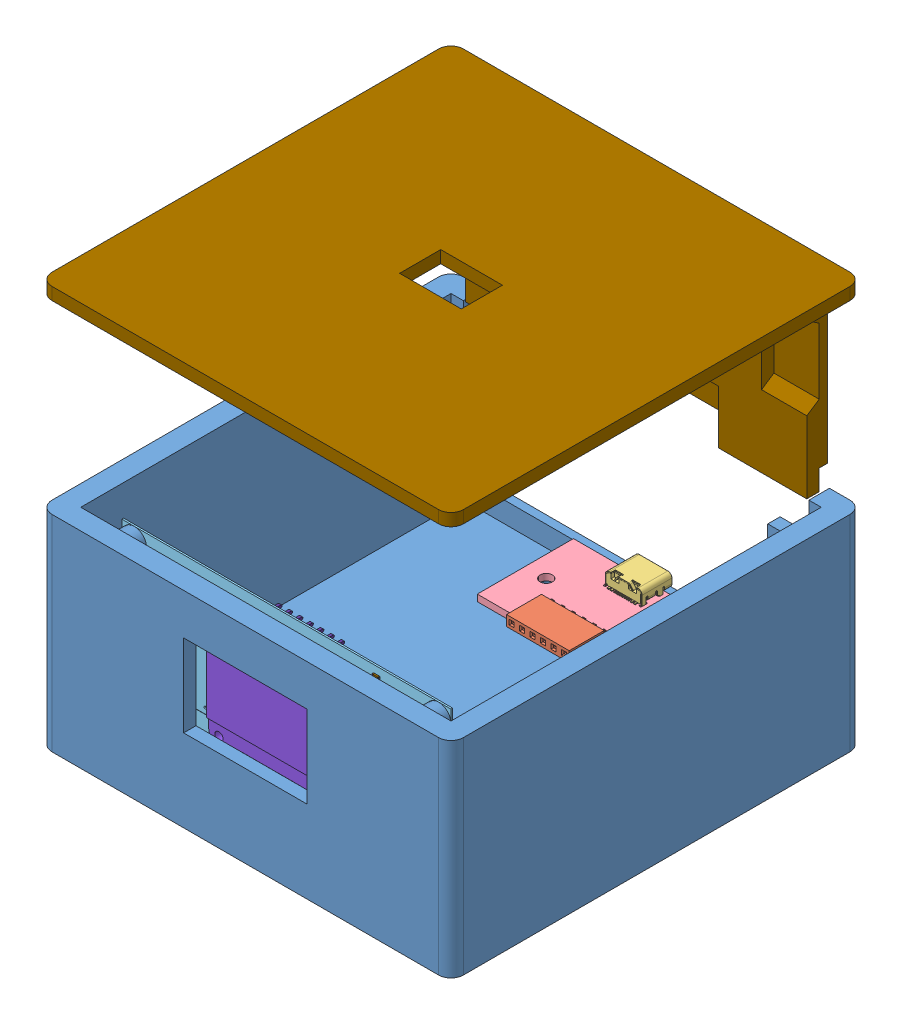
SolidWorks assembly 提醒喝水器, configuration 默认. Lengths in mm.
Overall size (100 98 100).
295 component instances, 117 part files, 15 mates.
Components (placement in the parent):
- 外壳-1: 外壳 [默认] at (-140.6896 -46.2345 50) size (100 50 100)
- Type-C_Ext-1: Type-C_Ext [默认] at (-1.1691 -37.2345 -151.062) x (0 0 1) z (0 1 0) size (28.17 35.81 6.47)
  - Type-C_Ext(2)^Type-C_Ext-1: Type-C_Ext(2)^Type-C_Ext [默认] at origin size (28.17 35.81 6.47) (virtual)
    - PinSocket_1x06_P2.54mm_Horizontal^Type-C_Ext(2)_Type-C_Ext-1: PinSocket_1x06_P2.54mm_Horizontal^Type-C_Ext(2)_Type-C_Ext [默认] at (120.06 -95.733 1.65) x (-1 0 0) z (0 0 1) size (10.13 15.24 5.84) (virtual)
      - SOLID^PinSocket_1x06_P2.54mm_Horizontal_Type-C_Ext(2)_Type-C_Ext-1: SOLID^PinSocket_1x06_P2.54mm_Horizontal_Type-C_Ext(2)_Type-C_Ext [默认] at origin size (10.13 15.24 5.84) (virtual)
    - Type-C_16Pin_ThroughtHole^Type-C_Ext(2)_Type-C_Ext-1: Type-C_16Pin_ThroughtHole^Type-C_Ext(2)_Type-C_Ext [默认] at (106.934 -89.408 0.126) x (0 -1 0) z (0 0 1) size (8.94 7.9 4.1) (virtual)
      - COMPOUND^Type-C_16Pin_ThroughtHole_Type-C_Ext(2)_Type-C_Ext-1: COMPOUND^Type-C_16Pin_ThroughtHole_Type-C_Ext(2)_Type-C_Ext [默认] at origin size (8.94 7.9 4.1) (virtual)
    - Type-C_Ext PCB^Type-C_Ext(2)_Type-C_Ext-1: Type-C_Ext PCB^Type-C_Ext(2)_Type-C_Ext [默认] at origin size (23.37 35.81 1.6) (virtual)
- MainBoard-1: MainBoard [默认] at (-130.6896 -38.7345 40) size (80 40 10.66)
  - MainBoard(2)^MainBoard-1: MainBoard(2)^MainBoard [默认] at origin size (80 40 10.66) (virtual)
    - Board^MainBoard(2)_MainBoard-1: Board^MainBoard(2)_MainBoard [默认] at origin size (80 40 0.41) (virtual)
      - Open CASCADE STEP translator 6.8 1.1.1^Board_MainBoard(2)_MainBoard-1: Open CASCADE STEP translator 6.8 1.1.1^Board_MainBoard(2)_MainBoard [默认] at (0 0 -0.4115) size (80 40 0.41) (virtual)
    - LS1^MainBoard(2)_MainBoard-1: LS1^MainBoard(2)_MainBoard [默认] at origin size (9 9 9) (virtual)
      - BEEP_5x9x5.5^LS1_MainBoard(2)_MainBoard-1: BEEP_5x9x5.5^LS1_MainBoard(2)_MainBoard [默认] at (40.0051 20.0659 -0.4115) x (1 0 0) z (0 0 -1) size (9 9 9) (virtual)
        - BEEP_5X9X5_5-3924_AF0_ASM^BEEP_5x9x5.5_LS1_MainBoard(2)_MainBoard-1: BEEP_5X9X5_5-3924_AF0_ASM^BEEP_5x9x5.5_LS1_MainBoard(2)_MainBoard [默认] at origin size (9 9 9) (virtual)
          - BEEP_5X9X5_5-6370_AF0^BEEP_5X9X5_5-3924_AF0_ASM_BEEP_5x9x5.5_LS1_MainBoard(2)_MainBoard-1: BEEP_5X9X5_5-6370_AF0^BEEP_5X9X5_5-3924_AF0_ASM_BEEP_5x9x5.5_LS1_MainBoard(2)_MainBoard [默认] at origin size (9 9 9) (virtual)
    - X1^MainBoard(2)_MainBoard-1: X1^MainBoard(2)_MainBoard [默认] at origin size (2.5 3.2 0.72) (virtual)
      - OSC_3225-4^X1_MainBoard(2)_MainBoard-1: OSC_3225-4^X1_MainBoard(2)_MainBoard [默认] at (73.6601 29.4639 0) x (0 -1 0) z (0 0 1) size (3.2 2.5 0.72) (virtual)
        - OSC_3225-4-6525_AF0_ASM^OSC_3225-4_X1_MainBoard(2)_MainBoard-1: OSC_3225-4-6525_AF0_ASM^OSC_3225-4_X1_MainBoard(2)_MainBoard [默认] at origin size (3.2 2.5 0.72) (virtual)
          - OSC_3225-4-11675_AF0_ASM^OSC_3225-4-6525_AF0_ASM_OSC_3225-4_X1_MainBoard(2)_MainBoard-1: OSC_3225-4-11675_AF0_ASM^OSC_3225-4-6525_AF0_ASM_OSC_3225-4_X1_MainBoard(2)_MainBoard [默认] at origin size (3.2 2.5 0.72) (virtual)
            - _3_1_20001^OSC_3225-4-11675_AF0_ASM_OSC_3225-4-6525_AF0_ASM_OSC_3225-4_X1_MainBoard(2)_MainBoard-1: _3_1_20001^OSC_3225-4-11675_AF0_ASM_OSC_3225-4-6525_AF0_ASM_OSC_3225-4_X1_MainBoard(2)_MainBoard [默认] at origin size (3.08 2.38 0.23) (virtual)
            - _4_4__1_20001^OSC_3225-4-11675_AF0_ASM_OSC_3225-4-6525_AF0_ASM_OSC_3225-4_X1_MainBoard(2)_MainBoard-1: _4_4__1_20001^OSC_3225-4-11675_AF0_ASM_OSC_3225-4-6525_AF0_ASM_OSC_3225-4_X1_MainBoard(2)_MainBoard [默认] at origin size (1 0.9 0.02) (virtual)
            - _4_2__1_20001^OSC_3225-4-11675_AF0_ASM_OSC_3225-4-6525_AF0_ASM_OSC_3225-4_X1_MainBoard(2)_MainBoard-1: _4_2__1_20001^OSC_3225-4-11675_AF0_ASM_OSC_3225-4-6525_AF0_ASM_OSC_3225-4_X1_MainBoard(2)_MainBoard [默认] at origin size (1 0.9 0.02) (virtual)
            - _4_1__1_20001^OSC_3225-4-11675_AF0_ASM_OSC_3225-4-6525_AF0_ASM_OSC_3225-4_X1_MainBoard(2)_MainBoard-1: _4_1__1_20001^OSC_3225-4-11675_AF0_ASM_OSC_3225-4-6525_AF0_ASM_OSC_3225-4_X1_MainBoard(2)_MainBoard [默认] at origin size (1 0.9 0.02) (virtual)
            - _4_3__1_20001^OSC_3225-4-11675_AF0_ASM_OSC_3225-4-6525_AF0_ASM_OSC_3225-4_X1_MainBoard(2)_MainBoard-1: _4_3__1_20001^OSC_3225-4-11675_AF0_ASM_OSC_3225-4-6525_AF0_ASM_OSC_3225-4_X1_MainBoard(2)_MainBoard [默认] at origin size (1 0.9 0.02) (virtual)
            - _2_1_2_AF0^OSC_3225-4-11675_AF0_ASM_OSC_3225-4-6525_AF0_ASM_OSC_3225-4_X1_MainBoard(2)_MainBoard-1: _2_1_2_AF0^OSC_3225-4-11675_AF0_ASM_OSC_3225-4-6525_AF0_ASM_OSC_3225-4_X1_MainBoard(2)_MainBoard [默认] at origin size (3.2 2.5 0.47) (virtual)
    - U2^MainBoard(2)_MainBoard-1: U2^MainBoard(2)_MainBoard [默认] at origin size (2.81 3 1.18) (virtual)
      - SOT23-6^U2_MainBoard(2)_MainBoard-1: SOT23-6^U2_MainBoard(2)_MainBoard [默认] at (55.1181 16.1291 0) x (0 -1 0) z (0 0 1) size (3 2.81 1.18) (virtual)
        - SOT23-6-13550_AF0_ASM^SOT23-6_U2_MainBoard(2)_MainBoard-1: SOT23-6-13550_AF0_ASM^SOT23-6_U2_MainBoard(2)_MainBoard [默认] at origin size (3 2.81 1.18) (virtual)
          - SOT23-5AND6__100^SOT23-6-13550_AF0_ASM_SOT23-6_U2_MainBoard(2)_MainBoard-1: SOT23-5AND6__100^SOT23-6-13550_AF0_ASM_SOT23-6_U2_MainBoard(2)_MainBoard [默认] at (0.95 0.8 0.675) size (0.4 0.6 0.78) (virtual)
          - SOT23-5AND6__100^SOT23-6-13550_AF0_ASM_SOT23-6_U2_MainBoard(2)_MainBoard-2: SOT23-5AND6__100^SOT23-6-13550_AF0_ASM_SOT23-6_U2_MainBoard(2)_MainBoard [默认] at (-0.95 -0.8 0.675) x (-1 0 0) z (0 0 1) size (0.4 0.6 0.78) (virtual)
          - SOT23-6-7933_AF0^SOT23-6-13550_AF0_ASM_SOT23-6_U2_MainBoard(2)_MainBoard-1: SOT23-6-7933_AF0^SOT23-6-13550_AF0_ASM_SOT23-6_U2_MainBoard(2)_MainBoard [默认] at origin size (3 1.6 1.1) (virtual)
          - SOT23-5AND6__100^SOT23-6-13550_AF0_ASM_SOT23-6_U2_MainBoard(2)_MainBoard-3: SOT23-5AND6__100^SOT23-6-13550_AF0_ASM_SOT23-6_U2_MainBoard(2)_MainBoard [默认] at (0 -0.8 0.675) x (-1 0 0) z (0 0 1) size (0.4 0.6 0.78) (virtual)
          - SOT23-5AND6__100^SOT23-6-13550_AF0_ASM_SOT23-6_U2_MainBoard(2)_MainBoard-4: SOT23-5AND6__100^SOT23-6-13550_AF0_ASM_SOT23-6_U2_MainBoard(2)_MainBoard [默认] at (0 0.8 0.675) size (0.4 0.6 0.78) (virtual)
          - SOT23-5AND6__100^SOT23-6-13550_AF0_ASM_SOT23-6_U2_MainBoard(2)_MainBoard-5: SOT23-5AND6__100^SOT23-6-13550_AF0_ASM_SOT23-6_U2_MainBoard(2)_MainBoard [默认] at (0.95 -0.8 0.675) x (-1 0 0) z (0 0 1) size (0.4 0.6 0.78) (virtual)
          - SOT23-5AND6__100^SOT23-6-13550_AF0_ASM_SOT23-6_U2_MainBoard(2)_MainBoard-6: SOT23-5AND6__100^SOT23-6-13550_AF0_ASM_SOT23-6_U2_MainBoard(2)_MainBoard [默认] at (-0.95 0.8 0.675) size (0.4 0.6 0.78) (virtual)
    - U1^MainBoard(2)_MainBoard-1: U1^MainBoard(2)_MainBoard [默认] at origin size (10.01 6.01 1.9) (virtual)
      - SOP16^U1_MainBoard(2)_MainBoard-1: SOP16^U1_MainBoard(2)_MainBoard [默认] at (65.913 29.7181 0) x (0 1 0) z (0 0 1) size (6.01 10.01 1.9) (virtual)
        - SOP16_1_AF0_ASM^SOP16_U1_MainBoard(2)_MainBoard-1: SOP16_1_AF0_ASM^SOP16_U1_MainBoard(2)_MainBoard [默认] at origin size (6.01 10.01 1.9) (virtual)
          - 1_8__10001^SOP16_1_AF0_ASM_SOP16_U1_MainBoard(2)_MainBoard-1: 1_8__10001^SOP16_1_AF0_ASM_SOP16_U1_MainBoard(2)_MainBoard [默认] at (-1.8 -4.44 1) x (0 -1 0) z (0 0 1) size (0.5 1.2 1.1) (virtual)
          - 1_8__10001^SOP16_1_AF0_ASM_SOP16_U1_MainBoard(2)_MainBoard-2: 1_8__10001^SOP16_1_AF0_ASM_SOP16_U1_MainBoard(2)_MainBoard [默认] at (1.8 -0.63 1) x (0 1 0) z (0 0 1) size (0.5 1.2 1.1) (virtual)
          - 1_8__10001^SOP16_1_AF0_ASM_SOP16_U1_MainBoard(2)_MainBoard-3: 1_8__10001^SOP16_1_AF0_ASM_SOP16_U1_MainBoard(2)_MainBoard [默认] at (-1.8 1.91 1) x (0 -1 0) z (0 0 1) size (0.5 1.2 1.1) (virtual)
          - SOP16__A^SOP16_1_AF0_ASM_SOP16_U1_MainBoard(2)_MainBoard-1: SOP16__A^SOP16_1_AF0_ASM_SOP16_U1_MainBoard(2)_MainBoard [默认] at origin size (3.61 10.01 1.8) (virtual)
          - 1_8__10001^SOP16_1_AF0_ASM_SOP16_U1_MainBoard(2)_MainBoard-4: 1_8__10001^SOP16_1_AF0_ASM_SOP16_U1_MainBoard(2)_MainBoard [默认] at (1.8 -1.9 1) x (0 1 0) z (0 0 1) size (0.5 1.2 1.1) (virtual)
          - 1_8__10001^SOP16_1_AF0_ASM_SOP16_U1_MainBoard(2)_MainBoard-5: 1_8__10001^SOP16_1_AF0_ASM_SOP16_U1_MainBoard(2)_MainBoard [默认] at (-1.8 0.64 1) x (0 -1 0) z (0 0 1) size (0.5 1.2 1.1) (virtual)
          - 1_8__10001^SOP16_1_AF0_ASM_SOP16_U1_MainBoard(2)_MainBoard-6: 1_8__10001^SOP16_1_AF0_ASM_SOP16_U1_MainBoard(2)_MainBoard [默认] at (1.8 4.45 1) x (0 1 0) z (0 0 1) size (0.5 1.2 1.1) (virtual)
          - 1_8__10001^SOP16_1_AF0_ASM_SOP16_U1_MainBoard(2)_MainBoard-7: 1_8__10001^SOP16_1_AF0_ASM_SOP16_U1_MainBoard(2)_MainBoard [默认] at (1.8 -3.17 1) x (0 1 0) z (0 0 1) size (0.5 1.2 1.1) (virtual)
          - 1_8__10001^SOP16_1_AF0_ASM_SOP16_U1_MainBoard(2)_MainBoard-8: 1_8__10001^SOP16_1_AF0_ASM_SOP16_U1_MainBoard(2)_MainBoard [默认] at (-1.8 -0.63 1) x (0 -1 0) z (0 0 1) size (0.5 1.2 1.1) (virtual)
          - 1_8__10001^SOP16_1_AF0_ASM_SOP16_U1_MainBoard(2)_MainBoard-9: 1_8__10001^SOP16_1_AF0_ASM_SOP16_U1_MainBoard(2)_MainBoard [默认] at (1.8 3.18 1) x (0 1 0) z (0 0 1) size (0.5 1.2 1.1) (virtual)
          - 1_8__10001^SOP16_1_AF0_ASM_SOP16_U1_MainBoard(2)_MainBoard-10: 1_8__10001^SOP16_1_AF0_ASM_SOP16_U1_MainBoard(2)_MainBoard [默认] at (1.8 -4.44 1) x (0 1 0) z (0 0 1) size (0.5 1.2 1.1) (virtual)
          - 1_8__10001^SOP16_1_AF0_ASM_SOP16_U1_MainBoard(2)_MainBoard-11: 1_8__10001^SOP16_1_AF0_ASM_SOP16_U1_MainBoard(2)_MainBoard [默认] at (-1.8 -1.9 1) x (0 -1 0) z (0 0 1) size (0.5 1.2 1.1) (virtual)
          - 1_8__10001^SOP16_1_AF0_ASM_SOP16_U1_MainBoard(2)_MainBoard-12: 1_8__10001^SOP16_1_AF0_ASM_SOP16_U1_MainBoard(2)_MainBoard [默认] at (1.8 1.91 1) x (0 1 0) z (0 0 1) size (0.5 1.2 1.1) (virtual)
          - 1_8__10001^SOP16_1_AF0_ASM_SOP16_U1_MainBoard(2)_MainBoard-13: 1_8__10001^SOP16_1_AF0_ASM_SOP16_U1_MainBoard(2)_MainBoard [默认] at (-1.8 4.45 1) x (0 -1 0) z (0 0 1) size (0.5 1.2 1.1) (virtual)
          - 1_8__10001^SOP16_1_AF0_ASM_SOP16_U1_MainBoard(2)_MainBoard-14: 1_8__10001^SOP16_1_AF0_ASM_SOP16_U1_MainBoard(2)_MainBoard [默认] at (-1.8 -3.17 1) x (0 -1 0) z (0 0 1) size (0.5 1.2 1.1) (virtual)
          - 1_8__10001^SOP16_1_AF0_ASM_SOP16_U1_MainBoard(2)_MainBoard-15: 1_8__10001^SOP16_1_AF0_ASM_SOP16_U1_MainBoard(2)_MainBoard [默认] at (1.8 0.64 1) x (0 1 0) z (0 0 1) size (0.5 1.2 1.1) (virtual)
          - 1_8__10001^SOP16_1_AF0_ASM_SOP16_U1_MainBoard(2)_MainBoard-16: 1_8__10001^SOP16_1_AF0_ASM_SOP16_U1_MainBoard(2)_MainBoard [默认] at (-1.8 3.18 1) x (0 -1 0) z (0 0 1) size (0.5 1.2 1.1) (virtual)
    - R11^MainBoard(2)_MainBoard-1: R11^MainBoard(2)_MainBoard [默认] at origin size (1.6 0.8 0.4) (virtual)
      - 0603^R11_MainBoard(2)_MainBoard-1: 0603^R11_MainBoard(2)_MainBoard [默认] at (53.213 12.0651 0) x (1 0 0) z (0 0 1) size (1.6 0.8 0.4) (virtual)
        - R_0603-3615_AF0_ASM^0603_R11_MainBoard(2)_MainBoard-1: R_0603-3615_AF0_ASM^0603_R11_MainBoard(2)_MainBoard [默认] at origin size (1.6 0.8 0.4) (virtual)
          - R_0603-3601_AF0_ASM^R_0603-3615_AF0_ASM_0603_R11_MainBoard(2)_MainBoard-1: R_0603-3601_AF0_ASM^R_0603-3615_AF0_ASM_0603_R11_MainBoard(2)_MainBoard [默认] at origin size (1.6 0.8 0.4) (virtual)
            - _2_1_2_3_4_5_60001^R_0603-3601_AF0_ASM_R_0603-3615_AF0_ASM_0603_R11_MainBoard(2)_MainBoard-1: _2_1_2_3_4_5_60001^R_0603-3601_AF0_ASM_R_0603-3615_AF0_ASM_0603_R11_MainBoard(2)_MainBoard [默认] at origin size (0.25 0.8 0.4) (virtual)
            - _7_1_2_3_AF0^R_0603-3601_AF0_ASM_R_0603-3615_AF0_ASM_0603_R11_MainBoard(2)_MainBoard-1: _7_1_2_3_AF0^R_0603-3601_AF0_ASM_R_0603-3615_AF0_ASM_0603_R11_MainBoard(2)_MainBoard [默认] at origin size (1.5 0.8 0.4) (virtual)
            - 5_1_2_3_4_5_600^R_0603-3601_AF0_ASM_R_0603-3615_AF0_ASM_0603_R11_MainBoard(2)_MainBoard-1: 5_1_2_3_4_5_600^R_0603-3601_AF0_ASM_R_0603-3615_AF0_ASM_0603_R11_MainBoard(2)_MainBoard [默认] at origin size (0.25 0.8 0.4) (virtual)
    - R10^MainBoard(2)_MainBoard-1: R10^MainBoard(2)_MainBoard [默认] at origin size (1.6 0.8 0.4) (virtual)
      - 0603^R10_MainBoard(2)_MainBoard-1: 0603^R10_MainBoard(2)_MainBoard [默认] at (58.928 14.9861 0) x (1 0 0) z (0 0 1) size (1.6 0.8 0.4) (virtual)
        - R_0603-3615_AF0_ASM^0603_R10_MainBoard(2)_MainBoard-1: R_0603-3615_AF0_ASM^0603_R10_MainBoard(2)_MainBoard [默认] at origin size (1.6 0.8 0.4) (virtual)
          - R_0603-3601_AF0_ASM^R_0603-3615_AF0_ASM_0603_R10_MainBoard(2)_MainBoard-1: R_0603-3601_AF0_ASM^R_0603-3615_AF0_ASM_0603_R10_MainBoard(2)_MainBoard [默认] at origin size (1.6 0.8 0.4) (virtual)
            - _2_1_2_3_4_5_60001^R_0603-3601_AF0_ASM_R_0603-3615_AF0_ASM_0603_R10_MainBoard(2)_MainBoard-1: _2_1_2_3_4_5_60001^R_0603-3601_AF0_ASM_R_0603-3615_AF0_ASM_0603_R10_MainBoard(2)_MainBoard [默认] at origin size (0.25 0.8 0.4) (virtual)
            - _7_1_2_3_AF0^R_0603-3601_AF0_ASM_R_0603-3615_AF0_ASM_0603_R10_MainBoard(2)_MainBoard-1: _7_1_2_3_AF0^R_0603-3601_AF0_ASM_R_0603-3615_AF0_ASM_0603_R10_MainBoard(2)_MainBoard [默认] at origin size (1.5 0.8 0.4) (virtual)
            - 5_1_2_3_4_5_600^R_0603-3601_AF0_ASM_R_0603-3615_AF0_ASM_0603_R10_MainBoard(2)_MainBoard-1: 5_1_2_3_4_5_600^R_0603-3601_AF0_ASM_R_0603-3615_AF0_ASM_0603_R10_MainBoard(2)_MainBoard [默认] at origin size (0.25 0.8 0.4) (virtual)
    - R9^MainBoard(2)_MainBoard-1: R9^MainBoard(2)_MainBoard [默认] at origin size (1.6 0.8 0.4) (virtual)
      - 0603^R9_MainBoard(2)_MainBoard-1: 0603^R9_MainBoard(2)_MainBoard [默认] at (53.2281 10.0332 0) x (1 0 0) z (0 0 1) size (1.6 0.8 0.4) (virtual)
        - R_0603-3615_AF0_ASM^0603_R9_MainBoard(2)_MainBoard-1: R_0603-3615_AF0_ASM^0603_R9_MainBoard(2)_MainBoard [默认] at origin size (1.6 0.8 0.4) (virtual)
          - R_0603-3601_AF0_ASM^R_0603-3615_AF0_ASM_0603_R9_MainBoard(2)_MainBoard-1: R_0603-3601_AF0_ASM^R_0603-3615_AF0_ASM_0603_R9_MainBoard(2)_MainBoard [默认] at origin size (1.6 0.8 0.4) (virtual)
            - _2_1_2_3_4_5_60001^R_0603-3601_AF0_ASM_R_0603-3615_AF0_ASM_0603_R9_MainBoard(2)_MainBoard-1: _2_1_2_3_4_5_60001^R_0603-3601_AF0_ASM_R_0603-3615_AF0_ASM_0603_R9_MainBoard(2)_MainBoard [默认] at origin size (0.25 0.8 0.4) (virtual)
            - _7_1_2_3_AF0^R_0603-3601_AF0_ASM_R_0603-3615_AF0_ASM_0603_R9_MainBoard(2)_MainBoard-1: _7_1_2_3_AF0^R_0603-3601_AF0_ASM_R_0603-3615_AF0_ASM_0603_R9_MainBoard(2)_MainBoard [默认] at origin size (1.5 0.8 0.4) (virtual)
            - 5_1_2_3_4_5_600^R_0603-3601_AF0_ASM_R_0603-3615_AF0_ASM_0603_R9_MainBoard(2)_MainBoard-1: 5_1_2_3_4_5_600^R_0603-3601_AF0_ASM_R_0603-3615_AF0_ASM_0603_R9_MainBoard(2)_MainBoard [默认] at origin size (0.25 0.8 0.4) (virtual)
    - R8^MainBoard(2)_MainBoard-1: R8^MainBoard(2)_MainBoard [默认] at origin size (1.6 0.8 0.4) (virtual)
      - 0603^R8_MainBoard(2)_MainBoard-1: 0603^R8_MainBoard(2)_MainBoard [默认] at (61.976 37.8461 0) x (1 0 0) z (0 0 1) size (1.6 0.8 0.4) (virtual)
        - R_0603-3615_AF0_ASM^0603_R8_MainBoard(2)_MainBoard-1: R_0603-3615_AF0_ASM^0603_R8_MainBoard(2)_MainBoard [默认] at origin size (1.6 0.8 0.4) (virtual)
          - R_0603-3601_AF0_ASM^R_0603-3615_AF0_ASM_0603_R8_MainBoard(2)_MainBoard-1: R_0603-3601_AF0_ASM^R_0603-3615_AF0_ASM_0603_R8_MainBoard(2)_MainBoard [默认] at origin size (1.6 0.8 0.4) (virtual)
            - _2_1_2_3_4_5_60001^R_0603-3601_AF0_ASM_R_0603-3615_AF0_ASM_0603_R8_MainBoard(2)_MainBoard-1: _2_1_2_3_4_5_60001^R_0603-3601_AF0_ASM_R_0603-3615_AF0_ASM_0603_R8_MainBoard(2)_MainBoard [默认] at origin size (0.25 0.8 0.4) (virtual)
            - _7_1_2_3_AF0^R_0603-3601_AF0_ASM_R_0603-3615_AF0_ASM_0603_R8_MainBoard(2)_MainBoard-1: _7_1_2_3_AF0^R_0603-3601_AF0_ASM_R_0603-3615_AF0_ASM_0603_R8_MainBoard(2)_MainBoard [默认] at origin size (1.5 0.8 0.4) (virtual)
            - 5_1_2_3_4_5_600^R_0603-3601_AF0_ASM_R_0603-3615_AF0_ASM_0603_R8_MainBoard(2)_MainBoard-1: 5_1_2_3_4_5_600^R_0603-3601_AF0_ASM_R_0603-3615_AF0_ASM_0603_R8_MainBoard(2)_MainBoard [默认] at origin size (0.25 0.8 0.4) (virtual)
    - R7^MainBoard(2)_MainBoard-1: R7^MainBoard(2)_MainBoard [默认] at origin size (0.8 1.6 0.4) (virtual)
      - 0603^R7_MainBoard(2)_MainBoard-1: 0603^R7_MainBoard(2)_MainBoard [默认] at (10.5411 7.62 0) x (0 -1 0) z (0 0 1) size (1.6 0.8 0.4) (virtual)
        - R_0603-3615_AF0_ASM^0603_R7_MainBoard(2)_MainBoard-1: R_0603-3615_AF0_ASM^0603_R7_MainBoard(2)_MainBoard [默认] at origin size (1.6 0.8 0.4) (virtual)
          - R_0603-3601_AF0_ASM^R_0603-3615_AF0_ASM_0603_R7_MainBoard(2)_MainBoard-1: R_0603-3601_AF0_ASM^R_0603-3615_AF0_ASM_0603_R7_MainBoard(2)_MainBoard [默认] at origin size (1.6 0.8 0.4) (virtual)
            - _2_1_2_3_4_5_60001^R_0603-3601_AF0_ASM_R_0603-3615_AF0_ASM_0603_R7_MainBoard(2)_MainBoard-1: _2_1_2_3_4_5_60001^R_0603-3601_AF0_ASM_R_0603-3615_AF0_ASM_0603_R7_MainBoard(2)_MainBoard [默认] at origin size (0.25 0.8 0.4) (virtual)
            - _7_1_2_3_AF0^R_0603-3601_AF0_ASM_R_0603-3615_AF0_ASM_0603_R7_MainBoard(2)_MainBoard-1: _7_1_2_3_AF0^R_0603-3601_AF0_ASM_R_0603-3615_AF0_ASM_0603_R7_MainBoard(2)_MainBoard [默认] at origin size (1.5 0.8 0.4) (virtual)
            - 5_1_2_3_4_5_600^R_0603-3601_AF0_ASM_R_0603-3615_AF0_ASM_0603_R7_MainBoard(2)_MainBoard-1: 5_1_2_3_4_5_600^R_0603-3601_AF0_ASM_R_0603-3615_AF0_ASM_0603_R7_MainBoard(2)_MainBoard [默认] at origin size (0.25 0.8 0.4) (virtual)
    - R6^MainBoard(2)_MainBoard-1: R6^MainBoard(2)_MainBoard [默认] at origin size (1.6 0.8 0.4) (virtual)
      - 0603^R6_MainBoard(2)_MainBoard-1: 0603^R6_MainBoard(2)_MainBoard [默认] at (61.976 35.8139 0) x (-1 0 0) z (0 0 1) size (1.6 0.8 0.4) (virtual)
        - R_0603-3615_AF0_ASM^0603_R6_MainBoard(2)_MainBoard-1: R_0603-3615_AF0_ASM^0603_R6_MainBoard(2)_MainBoard [默认] at origin size (1.6 0.8 0.4) (virtual)
          - R_0603-3601_AF0_ASM^R_0603-3615_AF0_ASM_0603_R6_MainBoard(2)_MainBoard-1: R_0603-3601_AF0_ASM^R_0603-3615_AF0_ASM_0603_R6_MainBoard(2)_MainBoard [默认] at origin size (1.6 0.8 0.4) (virtual)
            - _2_1_2_3_4_5_60001^R_0603-3601_AF0_ASM_R_0603-3615_AF0_ASM_0603_R6_MainBoard(2)_MainBoard-1: _2_1_2_3_4_5_60001^R_0603-3601_AF0_ASM_R_0603-3615_AF0_ASM_0603_R6_MainBoard(2)_MainBoard [默认] at origin size (0.25 0.8 0.4) (virtual)
            - _7_1_2_3_AF0^R_0603-3601_AF0_ASM_R_0603-3615_AF0_ASM_0603_R6_MainBoard(2)_MainBoard-1: _7_1_2_3_AF0^R_0603-3601_AF0_ASM_R_0603-3615_AF0_ASM_0603_R6_MainBoard(2)_MainBoard [默认] at origin size (1.5 0.8 0.4) (virtual)
            - 5_1_2_3_4_5_600^R_0603-3601_AF0_ASM_R_0603-3615_AF0_ASM_0603_R6_MainBoard(2)_MainBoard-1: 5_1_2_3_4_5_600^R_0603-3601_AF0_ASM_R_0603-3615_AF0_ASM_0603_R6_MainBoard(2)_MainBoard [默认] at origin size (0.25 0.8 0.4) (virtual)
    - R5^MainBoard(2)_MainBoard-1: R5^MainBoard(2)_MainBoard [默认] at origin size (1.6 0.8 0.4) (virtual)
      - 0603^R5_MainBoard(2)_MainBoard-1: 0603^R5_MainBoard(2)_MainBoard [默认] at (28.956 27.4321 0) x (1 0 0) z (0 0 1) size (1.6 0.8 0.4) (virtual)
        - R_0603-3615_AF0_ASM^0603_R5_MainBoard(2)_MainBoard-1: R_0603-3615_AF0_ASM^0603_R5_MainBoard(2)_MainBoard [默认] at origin size (1.6 0.8 0.4) (virtual)
          - R_0603-3601_AF0_ASM^R_0603-3615_AF0_ASM_0603_R5_MainBoard(2)_MainBoard-1: R_0603-3601_AF0_ASM^R_0603-3615_AF0_ASM_0603_R5_MainBoard(2)_MainBoard [默认] at origin size (1.6 0.8 0.4) (virtual)
            - _2_1_2_3_4_5_60001^R_0603-3601_AF0_ASM_R_0603-3615_AF0_ASM_0603_R5_MainBoard(2)_MainBoard-1: _2_1_2_3_4_5_60001^R_0603-3601_AF0_ASM_R_0603-3615_AF0_ASM_0603_R5_MainBoard(2)_MainBoard [默认] at origin size (0.25 0.8 0.4) (virtual)
            - _7_1_2_3_AF0^R_0603-3601_AF0_ASM_R_0603-3615_AF0_ASM_0603_R5_MainBoard(2)_MainBoard-1: _7_1_2_3_AF0^R_0603-3601_AF0_ASM_R_0603-3615_AF0_ASM_0603_R5_MainBoard(2)_MainBoard [默认] at origin size (1.5 0.8 0.4) (virtual)
            - 5_1_2_3_4_5_600^R_0603-3601_AF0_ASM_R_0603-3615_AF0_ASM_0603_R5_MainBoard(2)_MainBoard-1: 5_1_2_3_4_5_600^R_0603-3601_AF0_ASM_R_0603-3615_AF0_ASM_0603_R5_MainBoard(2)_MainBoard [默认] at origin size (0.25 0.8 0.4) (virtual)
    - R4^MainBoard(2)_MainBoard-1: R4^MainBoard(2)_MainBoard [默认] at origin size (0.8 1.6 0.4) (virtual)
      - 0603^R4_MainBoard(2)_MainBoard-1: 0603^R4_MainBoard(2)_MainBoard [默认] at (25.9077 5.207 0) x (0 1 0) z (0 0 1) size (1.6 0.8 0.4) (virtual)
        - R_0603-3615_AF0_ASM^0603_R4_MainBoard(2)_MainBoard-1: R_0603-3615_AF0_ASM^0603_R4_MainBoard(2)_MainBoard [默认] at origin size (1.6 0.8 0.4) (virtual)
          - R_0603-3601_AF0_ASM^R_0603-3615_AF0_ASM_0603_R4_MainBoard(2)_MainBoard-1: R_0603-3601_AF0_ASM^R_0603-3615_AF0_ASM_0603_R4_MainBoard(2)_MainBoard [默认] at origin size (1.6 0.8 0.4) (virtual)
            - _2_1_2_3_4_5_60001^R_0603-3601_AF0_ASM_R_0603-3615_AF0_ASM_0603_R4_MainBoard(2)_MainBoard-1: _2_1_2_3_4_5_60001^R_0603-3601_AF0_ASM_R_0603-3615_AF0_ASM_0603_R4_MainBoard(2)_MainBoard [默认] at origin size (0.25 0.8 0.4) (virtual)
            - _7_1_2_3_AF0^R_0603-3601_AF0_ASM_R_0603-3615_AF0_ASM_0603_R4_MainBoard(2)_MainBoard-1: _7_1_2_3_AF0^R_0603-3601_AF0_ASM_R_0603-3615_AF0_ASM_0603_R4_MainBoard(2)_MainBoard [默认] at origin size (1.5 0.8 0.4) (virtual)
            - 5_1_2_3_4_5_600^R_0603-3601_AF0_ASM_R_0603-3615_AF0_ASM_0603_R4_MainBoard(2)_MainBoard-1: 5_1_2_3_4_5_600^R_0603-3601_AF0_ASM_R_0603-3615_AF0_ASM_0603_R4_MainBoard(2)_MainBoard [默认] at origin size (0.25 0.8 0.4) (virtual)
    - R3^MainBoard(2)_MainBoard-1: R3^MainBoard(2)_MainBoard [默认] at origin size (1.6 0.8 0.4) (virtual)
      - 0603^R3_MainBoard(2)_MainBoard-1: 0603^R3_MainBoard(2)_MainBoard [默认] at (34.925 9.3979 0) x (-1 0 0) z (0 0 1) size (1.6 0.8 0.4) (virtual)
        - R_0603-3615_AF0_ASM^0603_R3_MainBoard(2)_MainBoard-1: R_0603-3615_AF0_ASM^0603_R3_MainBoard(2)_MainBoard [默认] at origin size (1.6 0.8 0.4) (virtual)
          - R_0603-3601_AF0_ASM^R_0603-3615_AF0_ASM_0603_R3_MainBoard(2)_MainBoard-1: R_0603-3601_AF0_ASM^R_0603-3615_AF0_ASM_0603_R3_MainBoard(2)_MainBoard [默认] at origin size (1.6 0.8 0.4) (virtual)
            - _2_1_2_3_4_5_60001^R_0603-3601_AF0_ASM_R_0603-3615_AF0_ASM_0603_R3_MainBoard(2)_MainBoard-1: _2_1_2_3_4_5_60001^R_0603-3601_AF0_ASM_R_0603-3615_AF0_ASM_0603_R3_MainBoard(2)_MainBoard [默认] at origin size (0.25 0.8 0.4) (virtual)
            - _7_1_2_3_AF0^R_0603-3601_AF0_ASM_R_0603-3615_AF0_ASM_0603_R3_MainBoard(2)_MainBoard-1: _7_1_2_3_AF0^R_0603-3601_AF0_ASM_R_0603-3615_AF0_ASM_0603_R3_MainBoard(2)_MainBoard [默认] at origin size (1.5 0.8 0.4) (virtual)
            - 5_1_2_3_4_5_600^R_0603-3601_AF0_ASM_R_0603-3615_AF0_ASM_0603_R3_MainBoard(2)_MainBoard-1: 5_1_2_3_4_5_600^R_0603-3601_AF0_ASM_R_0603-3615_AF0_ASM_0603_R3_MainBoard(2)_MainBoard [默认] at origin size (0.25 0.8 0.4) (virtual)
    - R2^MainBoard(2)_MainBoard-1: R2^MainBoard(2)_MainBoard [默认] at origin size (0.8 1.6 0.4) (virtual)
      - 0603^R2_MainBoard(2)_MainBoard-1: 0603^R2_MainBoard(2)_MainBoard [默认] at (45.3388 6.5891 0) x (0 1 0) z (0 0 1) size (1.6 0.8 0.4) (virtual)
        - R_0603-3615_AF0_ASM^0603_R2_MainBoard(2)_MainBoard-1: R_0603-3615_AF0_ASM^0603_R2_MainBoard(2)_MainBoard [默认] at origin size (1.6 0.8 0.4) (virtual)
          - R_0603-3601_AF0_ASM^R_0603-3615_AF0_ASM_0603_R2_MainBoard(2)_MainBoard-1: R_0603-3601_AF0_ASM^R_0603-3615_AF0_ASM_0603_R2_MainBoard(2)_MainBoard [默认] at origin size (1.6 0.8 0.4) (virtual)
            - _2_1_2_3_4_5_60001^R_0603-3601_AF0_ASM_R_0603-3615_AF0_ASM_0603_R2_MainBoard(2)_MainBoard-1: _2_1_2_3_4_5_60001^R_0603-3601_AF0_ASM_R_0603-3615_AF0_ASM_0603_R2_MainBoard(2)_MainBoard [默认] at origin size (0.25 0.8 0.4) (virtual)
            - _7_1_2_3_AF0^R_0603-3601_AF0_ASM_R_0603-3615_AF0_ASM_0603_R2_MainBoard(2)_MainBoard-1: _7_1_2_3_AF0^R_0603-3601_AF0_ASM_R_0603-3615_AF0_ASM_0603_R2_MainBoard(2)_MainBoard [默认] at origin size (1.5 0.8 0.4) (virtual)
            - 5_1_2_3_4_5_600^R_0603-3601_AF0_ASM_R_0603-3615_AF0_ASM_0603_R2_MainBoard(2)_MainBoard-1: 5_1_2_3_4_5_600^R_0603-3601_AF0_ASM_R_0603-3615_AF0_ASM_0603_R2_MainBoard(2)_MainBoard [默认] at origin size (0.25 0.8 0.4) (virtual)
    - R1^MainBoard(2)_MainBoard-1: R1^MainBoard(2)_MainBoard [默认] at origin size (1.6 0.8 0.4) (virtual)
      - 0603^R1_MainBoard(2)_MainBoard-1: 0603^R1_MainBoard(2)_MainBoard [默认] at (28.956 25.7811 0) x (1 0 0) z (0 0 1) size (1.6 0.8 0.4) (virtual)
        - R_0603-3615_AF0_ASM^0603_R1_MainBoard(2)_MainBoard-1: R_0603-3615_AF0_ASM^0603_R1_MainBoard(2)_MainBoard [默认] at origin size (1.6 0.8 0.4) (virtual)
          - R_0603-3601_AF0_ASM^R_0603-3615_AF0_ASM_0603_R1_MainBoard(2)_MainBoard-1: R_0603-3601_AF0_ASM^R_0603-3615_AF0_ASM_0603_R1_MainBoard(2)_MainBoard [默认] at origin size (1.6 0.8 0.4) (virtual)
            - _2_1_2_3_4_5_60001^R_0603-3601_AF0_ASM_R_0603-3615_AF0_ASM_0603_R1_MainBoard(2)_MainBoard-1: _2_1_2_3_4_5_60001^R_0603-3601_AF0_ASM_R_0603-3615_AF0_ASM_0603_R1_MainBoard(2)_MainBoard [默认] at origin size (0.25 0.8 0.4) (virtual)
            - _7_1_2_3_AF0^R_0603-3601_AF0_ASM_R_0603-3615_AF0_ASM_0603_R1_MainBoard(2)_MainBoard-1: _7_1_2_3_AF0^R_0603-3601_AF0_ASM_R_0603-3615_AF0_ASM_0603_R1_MainBoard(2)_MainBoard [默认] at origin size (1.5 0.8 0.4) (virtual)
            - 5_1_2_3_4_5_600^R_0603-3601_AF0_ASM_R_0603-3615_AF0_ASM_0603_R1_MainBoard(2)_MainBoard-1: 5_1_2_3_4_5_600^R_0603-3601_AF0_ASM_R_0603-3615_AF0_ASM_0603_R1_MainBoard(2)_MainBoard [默认] at origin size (0.25 0.8 0.4) (virtual)
    - Q3^MainBoard(2)_MainBoard-1: Q3^MainBoard(2)_MainBoard [默认] at origin size (2.4 3.01 1.05) (virtual)
      - SOT23-3-2^Q3_MainBoard(2)_MainBoard-1: SOT23-3-2^Q3_MainBoard(2)_MainBoard [默认] at (56.3879 31.1149 0) x (0 1 0) z (0 0 1) size (3.01 2.4 1.05) (virtual)
        - SOT23-3-8473_AF0_ASM^SOT23-3-2_Q3_MainBoard(2)_MainBoard-1: SOT23-3-8473_AF0_ASM^SOT23-3-2_Q3_MainBoard(2)_MainBoard [默认] at origin size (3.01 2.4 1.05) (virtual)
          - SOT23-3_00^SOT23-3-8473_AF0_ASM_SOT23-3-2_Q3_MainBoard(2)_MainBoard-1: SOT23-3_00^SOT23-3-8473_AF0_ASM_SOT23-3-2_Q3_MainBoard(2)_MainBoard [默认] at (-0.95 -0.5461 0.475) x (-1 0 0) z (0 0 1) size (0.4 0.65 0.55) (virtual)
          - SOT23-3_00^SOT23-3-8473_AF0_ASM_SOT23-3-2_Q3_MainBoard(2)_MainBoard-2: SOT23-3_00^SOT23-3-8473_AF0_ASM_SOT23-3-2_Q3_MainBoard(2)_MainBoard [默认] at (0.95 -0.5461 0.475) x (-1 0 0) z (0 0 1) size (0.4 0.65 0.55) (virtual)
          - SOT23-3-2892_AF0^SOT23-3-8473_AF0_ASM_SOT23-3-2_Q3_MainBoard(2)_MainBoard-1: SOT23-3-2892_AF0^SOT23-3-8473_AF0_ASM_SOT23-3-2_Q3_MainBoard(2)_MainBoard [默认] at origin size (3.01 1.31 1) (virtual)
          - SOT23-3_00^SOT23-3-8473_AF0_ASM_SOT23-3-2_Q3_MainBoard(2)_MainBoard-3: SOT23-3_00^SOT23-3-8473_AF0_ASM_SOT23-3-2_Q3_MainBoard(2)_MainBoard [默认] at (0 0.5461 0.475) size (0.4 0.65 0.55) (virtual)
    - Q2^MainBoard(2)_MainBoard-1: Q2^MainBoard(2)_MainBoard [默认] at origin size (2.4 3.01 1.05) (virtual)
      - SOT23-3-2^Q2_MainBoard(2)_MainBoard-1: SOT23-3-2^Q2_MainBoard(2)_MainBoard [默认] at (56.3879 34.9249 0) x (0 1 0) z (0 0 1) size (3.01 2.4 1.05) (virtual)
        - SOT23-3-8473_AF0_ASM^SOT23-3-2_Q2_MainBoard(2)_MainBoard-1: SOT23-3-8473_AF0_ASM^SOT23-3-2_Q2_MainBoard(2)_MainBoard [默认] at origin size (3.01 2.4 1.05) (virtual)
          - SOT23-3_00^SOT23-3-8473_AF0_ASM_SOT23-3-2_Q2_MainBoard(2)_MainBoard-1: SOT23-3_00^SOT23-3-8473_AF0_ASM_SOT23-3-2_Q2_MainBoard(2)_MainBoard [默认] at (-0.95 -0.5461 0.475) x (-1 0 0) z (0 0 1) size (0.4 0.65 0.55) (virtual)
          - SOT23-3_00^SOT23-3-8473_AF0_ASM_SOT23-3-2_Q2_MainBoard(2)_MainBoard-2: SOT23-3_00^SOT23-3-8473_AF0_ASM_SOT23-3-2_Q2_MainBoard(2)_MainBoard [默认] at (0.95 -0.5461 0.475) x (-1 0 0) z (0 0 1) size (0.4 0.65 0.55) (virtual)
          - SOT23-3-2892_AF0^SOT23-3-8473_AF0_ASM_SOT23-3-2_Q2_MainBoard(2)_MainBoard-1: SOT23-3-2892_AF0^SOT23-3-8473_AF0_ASM_SOT23-3-2_Q2_MainBoard(2)_MainBoard [默认] at origin size (3.01 1.31 1) (virtual)
          - SOT23-3_00^SOT23-3-8473_AF0_ASM_SOT23-3-2_Q2_MainBoard(2)_MainBoard-3: SOT23-3_00^SOT23-3-8473_AF0_ASM_SOT23-3-2_Q2_MainBoard(2)_MainBoard [默认] at (0 0.5461 0.475) size (0.4 0.65 0.55) (virtual)
    - Q1^MainBoard(2)_MainBoard-1: Q1^MainBoard(2)_MainBoard [默认] at origin size (3.01 2.4 1.05) (virtual)
      - SOT23-3-2^Q1_MainBoard(2)_MainBoard-1: SOT23-3-2^Q1_MainBoard(2)_MainBoard [默认] at (29.4639 5.5881 0) x (1 0 0) z (0 0 1) size (3.01 2.4 1.05) (virtual)
        - SOT23-3-8473_AF0_ASM^SOT23-3-2_Q1_MainBoard(2)_MainBoard-1: SOT23-3-8473_AF0_ASM^SOT23-3-2_Q1_MainBoard(2)_MainBoard [默认] at origin size (3.01 2.4 1.05) (virtual)
          - SOT23-3_00^SOT23-3-8473_AF0_ASM_SOT23-3-2_Q1_MainBoard(2)_MainBoard-1: SOT23-3_00^SOT23-3-8473_AF0_ASM_SOT23-3-2_Q1_MainBoard(2)_MainBoard [默认] at (-0.95 -0.5461 0.475) x (-1 0 0) z (0 0 1) size (0.4 0.65 0.55) (virtual)
          - SOT23-3_00^SOT23-3-8473_AF0_ASM_SOT23-3-2_Q1_MainBoard(2)_MainBoard-2: SOT23-3_00^SOT23-3-8473_AF0_ASM_SOT23-3-2_Q1_MainBoard(2)_MainBoard [默认] at (0.95 -0.5461 0.475) x (-1 0 0) z (0 0 1) size (0.4 0.65 0.55) (virtual)
          - SOT23-3-2892_AF0^SOT23-3-8473_AF0_ASM_SOT23-3-2_Q1_MainBoard(2)_MainBoard-1: SOT23-3-2892_AF0^SOT23-3-8473_AF0_ASM_SOT23-3-2_Q1_MainBoard(2)_MainBoard [默认] at origin size (3.01 1.31 1) (virtual)
          - SOT23-3_00^SOT23-3-8473_AF0_ASM_SOT23-3-2_Q1_MainBoard(2)_MainBoard-3: SOT23-3_00^SOT23-3-8473_AF0_ASM_SOT23-3-2_Q1_MainBoard(2)_MainBoard [默认] at (0 0.5461 0.475) size (0.4 0.65 0.55) (virtual)
    - MD1^MainBoard(2)_MainBoard-1: MD1^MainBoard(2)_MainBoard [默认] at origin size (25.5 18 3.2) (virtual)
      - UNK_Espressif_Systems_ESP32-WROOM-32D_eec^MD1_MainBoard(2)_MainBoard-1: UNK_Espressif_Systems_ESP32-WROOM-32D_eec^MD1_MainBoard(2)_MainBoard [默认] at (13 20 0) x (0 1 0) z (0 0 1) size (18 25.5 3.2) (virtual)
        - pcb^UNK_Espressif_Systems_ESP32-WROOM-32D_eec_MD1_MainBoard(2)_MainBoard-1: pcb^UNK_Espressif_Systems_ESP32-WROOM-32D_eec_MD1_MainBoard(2)_MainBoard [默认] at origin size (18 25.5 0.9) (virtual)
        - pads^UNK_Espressif_Systems_ESP32-WROOM-32D_eec_MD1_MainBoard(2)_MainBoard-1: pads^UNK_Espressif_Systems_ESP32-WROOM-32D_eec_MD1_MainBoard(2)_MainBoard [默认] at origin size (18 19.8 0.91) (virtual)
        - antenna^UNK_Espressif_Systems_ESP32-WROOM-32D_eec_MD1_MainBoard(2)_MainBoard-1: antenna^UNK_Espressif_Systems_ESP32-WROOM-32D_eec_MD1_MainBoard(2)_MainBoard [默认] at (0 0 0.9) size (15.2 5.77 0) (virtual)
        - shell^UNK_Espressif_Systems_ESP32-WROOM-32D_eec_MD1_MainBoard(2)_MainBoard-1: shell^UNK_Espressif_Systems_ESP32-WROOM-32D_eec_MD1_MainBoard(2)_MainBoard [默认] at (0 0 0.9) size (15.8 17.6 2.3) (virtual)
        - logo^UNK_Espressif_Systems_ESP32-WROOM-32D_eec_MD1_MainBoard(2)_MainBoard-1: logo^UNK_Espressif_Systems_ESP32-WROOM-32D_eec_MD1_MainBoard(2)_MainBoard [默认] at (0 -3.09 3.2) size (12.19 6.06 0) (virtual)
    - L1^MainBoard(2)_MainBoard-1: L1^MainBoard(2)_MainBoard [默认] at origin size (3.21 1.61 0.91) (virtual)
      - L1206^L1_MainBoard(2)_MainBoard-1: L1206^L1_MainBoard(2)_MainBoard [默认] at (54.864 22.0981 0) x (1 0 0) z (0 0 1) size (3.21 1.6 0.91) (virtual)
        - 1206-157_AF0_ASM^L1206_L1_MainBoard(2)_MainBoard-1: 1206-157_AF0_ASM^L1206_L1_MainBoard(2)_MainBoard [默认] at origin size (3.21 1.6 0.91) (virtual)
          - 1206-7095_AF0_ASM^1206-157_AF0_ASM_L1206_L1_MainBoard(2)_MainBoard-1: 1206-7095_AF0_ASM^1206-157_AF0_ASM_L1206_L1_MainBoard(2)_MainBoard [默认] x (1 0 0) z (0 -1 0) size (3.21 0.91 1.6) (virtual)
            - 5_1_2_3_400^1206-7095_AF0_ASM_1206-157_AF0_ASM_L1206_L1_MainBoard(2)_MainBoard-1: 5_1_2_3_400^1206-7095_AF0_ASM_1206-157_AF0_ASM_L1206_L1_MainBoard(2)_MainBoard [默认] at origin size (0.5 0.91 1.6) (virtual)
            - 4_1_2_3_4_500^1206-7095_AF0_ASM_1206-157_AF0_ASM_L1206_L1_MainBoard(2)_MainBoard-1: 4_1_2_3_4_500^1206-7095_AF0_ASM_1206-157_AF0_ASM_L1206_L1_MainBoard(2)_MainBoard [默认] at origin size (0.5 0.91 1.6) (virtual)
            - _3_1_2_3_4_AF0^1206-7095_AF0_ASM_1206-157_AF0_ASM_L1206_L1_MainBoard(2)_MainBoard-1: _3_1_2_3_4_AF0^1206-7095_AF0_ASM_1206-157_AF0_ASM_L1206_L1_MainBoard(2)_MainBoard [默认] at origin size (2.2 0.9 1.6) (virtual)
    - JP4^MainBoard(2)_MainBoard-1: JP4^MainBoard(2)_MainBoard [默认] at origin size (7.54 5.7 9.5) (virtual)
      - XH2.54-2P^JP4_MainBoard(2)_MainBoard-1: XH2.54-2P^JP4_MainBoard(2)_MainBoard [默认] at (41.148 5.461 -0.4615) x (-1 0 0) z (0 -1 0) size (7.54 9.5 5.7) (virtual)
        - XH2.54-2P-0^XH2.54-2P_JP4_MainBoard(2)_MainBoard-1: XH2.54-2P-0^XH2.54-2P_JP4_MainBoard(2)_MainBoard [默认] at origin size (7.54 9.5 5.7) (virtual)
        - LOGO_^XH2.54-2P_JP4_MainBoard(2)_MainBoard-1: LOGO_^XH2.54-2P_JP4_MainBoard(2)_MainBoard [默认] at (-1.7013 -0.001 0) x (0 0 1) z (0 -1 0) size (0.9 1.04 0.01) (virtual)
    - JP2^MainBoard(2)_MainBoard-1: JP2^MainBoard(2)_MainBoard [默认] at origin size (17.7 5.7 9.5) (virtual)
      - XH2.54-6P^JP2_MainBoard(2)_MainBoard-1: XH2.54-6P^JP2_MainBoard(2)_MainBoard [默认] at (73.787 5.588 -0.4415) x (-1 0 0) z (0 -1 0) size (17.7 9.5 5.7) (virtual)
        - LOGO_-3^XH2.54-6P_JP2_MainBoard(2)_MainBoard-1: LOGO_-3^XH2.54-6P_JP2_MainBoard(2)_MainBoard [默认] at (-1.7013 -0.001 0) x (0 0 1) z (0 -1 0) size (0.9 1.04 0.01) (virtual)
        - XH2.54-6P-4^XH2.54-6P_JP2_MainBoard(2)_MainBoard-1: XH2.54-6P-4^XH2.54-6P_JP2_MainBoard(2)_MainBoard [默认] at origin size (17.7 9.5 5.7) (virtual)
    - JP1^MainBoard(2)_MainBoard-1: JP1^MainBoard(2)_MainBoard [默认] at origin size (2.54 2.4 7.2) (virtual)
      - HDR1_27-LI-2P^JP1_MainBoard(2)_MainBoard-1: HDR1_27-LI-2P^JP1_MainBoard(2)_MainBoard [默认] at (28.956 29.7179 -0.4115) x (1 0 0) z (0 0 -1) size (2.54 2.4 7.2) (virtual)
        - HDR1_27-LI-2P_1_AF0_ASM^HDR1_27-LI-2P_JP1_MainBoard(2)_MainBoard-1: HDR1_27-LI-2P_1_AF0_ASM^HDR1_27-LI-2P_JP1_MainBoard(2)_MainBoard [默认] at origin size (2.54 2.4 7.2) (virtual)
          - HDR1_27-LI-1P^HDR1_27-LI-2P_1_AF0_ASM_HDR1_27-LI-2P_JP1_MainBoard(2)_MainBoard-1: HDR1_27-LI-1P^HDR1_27-LI-2P_1_AF0_ASM_HDR1_27-LI-2P_JP1_MainBoard(2)_MainBoard [默认] at (-0.635 0 0) size (1.27 2.4 7.2) (virtual)
          - HDR1_27-LI-1P_AF0^HDR1_27-LI-2P_1_AF0_ASM_HDR1_27-LI-2P_JP1_MainBoard(2)_MainBoard-1: HDR1_27-LI-1P_AF0^HDR1_27-LI-2P_1_AF0_ASM_HDR1_27-LI-2P_JP1_MainBoard(2)_MainBoard [默认] at (0.635 0 0) size (1.27 2.4 7.2) (virtual)
    - D2^MainBoard(2)_MainBoard-1: D2^MainBoard(2)_MainBoard [默认] at origin size (1.6 0.8 0.61) (virtual)
      - LED_0603-R^D2_MainBoard(2)_MainBoard-1: LED_0603-R^D2_MainBoard(2)_MainBoard [默认] at (39.878 9.398 0) x (-1 0 0) z (0 0 1) size (1.6 0.8 0.47) (virtual)
